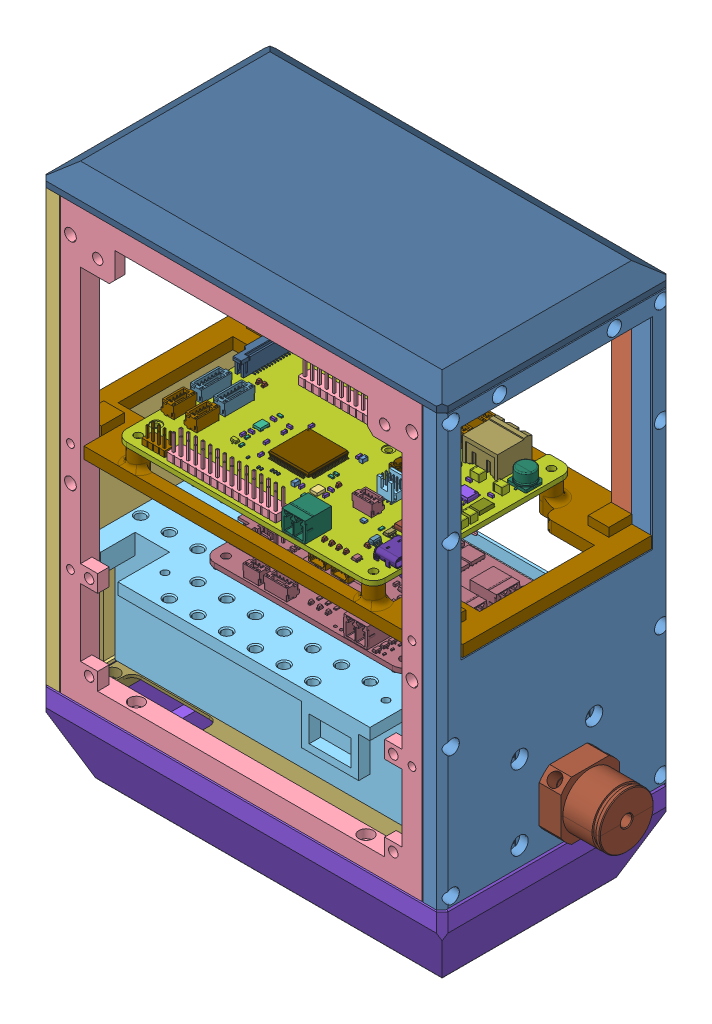
SolidWorks assembly twipr, configuration Default. Lengths in mm. (continued)
Components (placement in the parent): (continued)
- robot-hub-1: robot-hub [Default] at (-323.8774 211.7203 115.5) x (-1 0 0) z (0 1 0) size (91.46 70 13.31) (continued)
  - robot-hub.step-1: robot-hub.step [Default] at origin size (91.46 70 13.31) (continued)
    - R_0603_1608Metric.step-39: R_0603_1608Metric.step [Default] at (94.4 -135.4 -0.05) x (0 -1 0) z (0 0 -1) size (1.6 0.8 0.45) (continued)
      - SOLID.step-1: SOLID.step [Default] at origin size (1.6 0.8 0.45)
    - C_1210_3225Metric.step-7: C_1210_3225Metric.step [Default] at (104.4 -92 -0.05) x (-1 0 0) z (0 0 -1) size (3.2 2.5 2.5)
      - SOLID-0.step-1: SOLID-0.step [Default] at origin size (3.2 2.5 2.5)
    - SOT-323_SC-70.step-3: SOT-323_SC-70.step [Default] at (97 -134 -0.05) x (1 0 0) z (0 0 -1) size (2 2 1.05)
      - SOLID-17.step-1: SOLID-17.step [Default] at origin size (2 2 1.05)
    - SM04B-SRSS-TB_dark.step-2: SM04B-SRSS-TB_dark.step [Default] at (159.3 -135.7 0.2) x (0 -1 0) z (1 0 0) size (6 2.96 4.95)
      - SOLID-37.step-1: SOLID-37.step [Default] at origin size (6 2.96 4.95)
    - C_0603_1608Metric.step-24: C_0603_1608Metric.step [Default] at (116.8 -86.6 -0.05) x (0 -1 0) z (0 0 -1) size (1.6 0.8 0.8)
      - SOLID-1.step-1: SOLID-1.step [Default] at origin size (1.6 0.8 0.8)
    - C_0603_1608Metric.step-25: C_0603_1608Metric.step [Default] at (137.5 -140.9 -0.05) x (0 1 0) z (0 0 -1) size (1.6 0.8 0.8)
      - SOLID-1.step-1: SOLID-1.step [Default] at origin size (1.6 0.8 0.8)
    - C_0805_2012Metric.step-7: C_0805_2012Metric.step [Default] at (85.7 -87.2 -0.05) x (1 0 0) z (0 0 -1) size (2 1.25 1.25)
      - SOLID-11.step-1: SOLID-11.step [Default] at origin size (2 1.25 1.25)
    - IS25LP032D-JNLA3-TR.step-2: IS25LP032D-JNLA3-TR.step [Default] at (144.7 -137.5 -0.05) x (0 -1 0) z (0 0 -1) size (6 4.9 1.75)
      - COMPOUND-21.step-1: COMPOUND-21.step [Default] at origin size (6 4.9 1.75)
    - C_0603_1608Metric.step-26: C_0603_1608Metric.step [Default] at (128 -105.5 -0.05) x (0 1 0) z (0 0 -1) size (1.6 0.8 0.8)
      - SOLID-1.step-1: SOLID-1.step [Default] at origin size (1.6 0.8 0.8)
    - SOT-23-6.step-2: SOT-23-6.step [Default] at (102.8 -123.7 -0.05) x (-1 0 0) z (0 0 -1) size (2.8 2.9 1.55)
      - SOLID-24.step-1: SOLID-24.step [Default] at origin size (2.8 2.9 1.55)
    - PCT2075TP,147.step-1: PCT2075TP,147.step [Default] at (116 -141.3 -0.05) x (0 -1 0) z (0 0 -1) size (3.1 2 0.8)
      - COMPOUND-44.step-1: COMPOUND-44.step [Default] at origin size (3.1 2 0.8)
    - sk6812_side.step-1: sk6812_side.step [Default] at (75.35 -89.1 -1.05) x (0 -1 0) z (-1 0 0) size (4 2 1.6)
      - SOLID-45.step-1: SOLID-45.step [Default] at origin size (4 2 1.6)
    - R_0603_1608Metric.step-40: R_0603_1608Metric.step [Default] at (96 -111.5 -0.05) x (1 0 0) z (0 0 -1) size (1.6 0.8 0.45)
      - SOLID.step-1: SOLID.step [Default] at origin size (1.6 0.8 0.45)
    - R_0603_1608Metric.step-41: R_0603_1608Metric.step [Default] at (77.2 -90.65 -0.05) x (0 1 0) z (0 0 -1) size (1.6 0.8 0.45)
      - SOLID.step-1: SOLID.step [Default] at origin size (1.6 0.8 0.45)
    - C_0603_1608Metric.step-27: C_0603_1608Metric.step [Default] at (105.3 -137.6 -0.05) x (0 1 0) z (0 0 -1) size (1.6 0.8 0.8)
      - SOLID-1.step-1: SOLID-1.step [Default] at origin size (1.6 0.8 0.8)
    - STM32G031G6U6.step-2: STM32G031G6U6.step [Default] at (108.7 -137.5 -0.05) x (1 0 0) z (0 0 -1) size (4.1 4.1 0.6)
      - COMPOUND-31.step-1: COMPOUND-31.step [Default] at origin size (4.1 4.1 0.6)
    - SN74LVC3G17DCTR.step-1: SN74LVC3G17DCTR.step [Default] at (134.75 -142.2 -0.05) x (0 1 0) z (0 0 -1) size (4 2.95 1.3)
      - COMPOUND-46.step-1: COMPOUND-46.step [Default] at origin size (4 2.95 1.3)
    - R_0603_1608Metric.step-42: R_0603_1608Metric.step [Default] at (108.9 -109.7 -0.05) x (-1 0 0) z (0 0 -1) size (1.6 0.8 0.45)
      - SOLID.step-1: SOLID.step [Default] at origin size (1.6 0.8 0.45)
    - C_0805_2012Metric.step-8: C_0805_2012Metric.step [Default] at (94.8 -100.9 -0.05) x (0 1 0) z (0 0 -1) size (2 1.25 1.25)
      - SOLID-11.step-1: SOLID-11.step [Default] at origin size (2 1.25 1.25)
    - M24512-DFDW6TP.step-2: M24512-DFDW6TP.step [Default] at (121.95 -141.55 -0.05) x (1 0 0) z (0 0 -1) size (6.4 3 1.2)
      - COMPOUND-38.step-1: COMPOUND-38.step [Default] at origin size (6.4 3 1.2)
    - C_0603_1608Metric.step-28: C_0603_1608Metric.step [Default] at (101.6 -87.75 -0.05) x (1 0 0) z (0 0 -1) size (1.6 0.8 0.8)
      - SOLID-1.step-1: SOLID-1.step [Default] at origin size (1.6 0.8 0.8)
    - C_0603_1608Metric.step-29: C_0603_1608Metric.step [Default] at (108 -133.3 -0.05) x (0 -1 0) z (0 0 -1) size (1.6 0.8 0.8)
      - SOLID-1.step-1: SOLID-1.step [Default] at origin size (1.6 0.8 0.8)
    - R_0603_1608Metric.step-43: R_0603_1608Metric.step [Default] at (126.9 -130.4 -0.05) x (0 -1 0) z (0 0 -1) size (1.6 0.8 0.45)
      - SOLID.step-1: SOLID.step [Default] at origin size (1.6 0.8 0.45)
    - R_0603_1608Metric.step-44: R_0603_1608Metric.step [Default] at (141.135 -134.9385 -0.05) x (0 1 0) z (0 0 -1) size (1.6 0.8 0.45)
      - SOLID.step-1: SOLID.step [Default] at origin size (1.6 0.8 0.45)
    - SOT-23-6.step-3: SOT-23-6.step [Default] at (153.1 -91.8 -0.05) x (1 0 0) z (0 0 -1) size (2.8 2.9 1.55)
      - SOLID-24.step-1: SOLID-24.step [Default] at origin size (2.8 2.9 1.55)
    - R_0603_1608Metric.step-45: R_0603_1608Metric.step [Default] at (119.59 -119.2 -0.05) x (-1 0 0) z (0 0 -1) size (1.6 0.8 0.45)
      - SOLID.step-1: SOLID.step [Default] at origin size (1.6 0.8 0.45)
    - R_0603_1608Metric.step-46: R_0603_1608Metric.step [Default] at (128.5 -130.4 -0.05) x (0 -1 0) z (0 0 -1) size (1.6 0.8 0.45)
      - SOLID.step-1: SOLID.step [Default] at origin size (1.6 0.8 0.45)
    - R_0603_1608Metric.step-47: R_0603_1608Metric.step [Default] at (128.8 -109 -0.05) x (0 1 0) z (0 0 -1) size (1.6 0.8 0.45)
      - SOLID.step-1: SOLID.step [Default] at origin size (1.6 0.8 0.45)
    - C_0805_2012Metric.step-9: C_0805_2012Metric.step [Default] at (96.9 -100.9 -0.05) x (0 1 0) z (0 0 -1) size (2 1.25 1.25)
      - SOLID-11.step-1: SOLID-11.step [Default] at origin size (2 1.25 1.25)
    - R_0603_1608Metric.step-48: R_0603_1608Metric.step [Default] at (141.135 -138.0385 -0.05) x (0 -1 0) z (0 0 -1) size (1.6 0.8 0.45)
      - SOLID.step-1: SOLID.step [Default] at origin size (1.6 0.8 0.45)
    - SM04B-SRSS-TB_dark.step-3: SM04B-SRSS-TB_dark.step [Default] at (101.5 -142.1 0.2) x (-1 0 0) z (0 -1 0) size (6 2.96 4.95)
      - SOLID-37.step-1: SOLID-37.step [Default] at origin size (6 2.96 4.95)
    - C_0603_1608Metric.step-30: C_0603_1608Metric.step [Default] at (139.0125 -133.3 -0.05) x (0 1 0) z (0 0 -1) size (1.6 0.8 0.8)
      - SOLID-1.step-1: SOLID-1.step [Default] at origin size (1.6 0.8 0.8)
    - R_0603_1608Metric.step-49: R_0603_1608Metric.step [Default] at (152.7 -142.2 -0.05) x (1 0 0) z (0 0 -1) size (1.6 0.8 0.45)
      - SOLID.step-1: SOLID.step [Default] at origin size (1.6 0.8 0.45)
    - C_0805_2012Metric.step-10: C_0805_2012Metric.step [Default] at (85.75 -93.75 -0.05) x (1 0 0) z (0 0 -1) size (2 1.25 1.25)
      - SOLID-11.step-1: SOLID-11.step [Default] at origin size (2 1.25 1.25)
    - R_0603_1608Metric.step-50: R_0603_1608Metric.step [Default] at (127.7 -96.9 -0.05) x (1 0 0) z (0 0 -1) size (1.6 0.8 0.45)
      - SOLID.step-1: SOLID.step [Default] at origin size (1.6 0.8 0.45)
    - C_0805_2012Metric.step-11: C_0805_2012Metric.step [Default] at (100.75 -132.4 -0.05) x (1 0 0) z (0 0 -1) size (2 1.25 1.25)
      - SOLID-11.step-1: SOLID-11.step [Default] at origin size (2 1.25 1.25)
    - NCV8187AMLE330TCG.step-1: NCV8187AMLE330TCG.step [Default] at (96.2 -119.9 -0.05) x (-1 0 0) z (0 0 -1) size (3.1 3 1)
      - COMPOUND-47.step-1: COMPOUND-47.step [Default] at origin size (3.1 3 1)
    - R_0402_1005Metric.step-11: R_0402_1005Metric.step [Default] at (91.95 -87.35 -0.05) x (-1 0 0) z (0 0 -1) size (1 0.5 0.35)
      - SOLID-3.step-1: SOLID-3.step [Default] at origin size (1 0.5 0.35)
    - SOIC-16_3.9x9.9mm_P1.27mm.step-1: SOIC-16_3.9x9.9mm_P1.27mm.step [Default] at (96.9 -106.7 -0.05) x (0 1 0) z (0 0 -1) size (6 9.9 1.75)
      - SOLID-48.step-1: SOLID-48.step [Default] at origin size (6 9.9 1.75)
    - C_0603_1608Metric.step-31: C_0603_1608Metric.step [Default] at (96.8 -92.75 -0.05) x (-1 0 0) z (0 0 -1) size (1.6 0.8 0.8)
      - SOLID-1.step-1: SOLID-1.step [Default] at origin size (1.6 0.8 0.8)
    - R_0603_1608Metric.step-51: R_0603_1608Metric.step [Default] at (107.7 -107.2 -0.05) x (0 1 0) z (0 0 -1) size (1.6 0.8 0.45)
      - SOLID.step-1: SOLID.step [Default] at origin size (1.6 0.8 0.45)
    - R_0603_1608Metric.step-52: R_0603_1608Metric.step [Default] at (141.5 -130.7 -0.05) x (0 -1 0) z (0 0 -1) size (1.6 0.8 0.45)
      - SOLID.step-1: SOLID.step [Default] at origin size (1.6 0.8 0.45)
    - ECS-120-20-33-CKM-TR.step-1: ECS-120-20-33-CKM-TR.step [Default] at (104.7 -102.5 -0.05) x (0 1 0) z (0 0 -1) size (3.38 2.68 0.9)
      - COMPOUND-49.step-1: COMPOUND-49.step [Default] at origin size (3.38 2.68 0.9)
    - R_0603_1608Metric.step-53: R_0603_1608Metric.step [Default] at (93.5 -139.3 -0.05) x (0 -1 0) z (0 0 -1) size (1.6 0.8 0.45)
      - SOLID.step-1: SOLID.step [Default] at origin size (1.6 0.8 0.45)
    - C_0603_1608Metric.step-32: C_0603_1608Metric.step [Default] at (125.4 -99.5 -0.05) x (0 1 0) z (0 0 -1) size (1.6 0.8 0.8)
      - SOLID-1.step-1: SOLID-1.step [Default] at origin size (1.6 0.8 0.8)
    - R_0402_1005Metric.step-12: R_0402_1005Metric.step [Default] at (91.95 -88.35 -0.05) x (1 0 0) z (0 0 -1) size (1 0.5 0.35)
      - SOLID-3.step-1: SOLID-3.step [Default] at origin size (1 0.5 0.35)
    - 5033981892.step-1: 5033981892.step [Default] at (97.05 29.65 -154.55) x (0 -1 0) z (0 0 1) size (13.1 14.05 1.28)
      - COMPOUND-50.step-1: COMPOUND-50.step [Default] at origin size (13.1 14.05 1.28)
    - R_0603_1608Metric.step-54: R_0603_1608Metric.step [Default] at (131.9625 -136.35 -0.05) x (0 -1 0) z (0 0 -1) size (1.6 0.8 0.45)
      - SOLID.step-1: SOLID.step [Default] at origin size (1.6 0.8 0.45)
    - SOT-563.step-2: SOT-563.step [Default] at (89.5 -84.65 -0.05) x (-1 0 0) z (0 0 -1) size (1.6 1.6 0.63)
      - SOLID-29.step-1: SOLID-29.step [Default] at origin size (1.6 1.6 0.63)
    - R_0603_1608Metric.step-55: R_0603_1608Metric.step [Default] at (94.45 -93.2 -0.05) x (0 -1 0) z (0 0 -1) size (1.6 0.8 0.45)
      - SOLID.step-1: SOLID.step [Default] at origin size (1.6 0.8 0.45)
    - R_0603_1608Metric.step-56: R_0603_1608Metric.step [Default] at (123.9 -130.4 -0.05) x (0 -1 0) z (0 0 -1) size (1.6 0.8 0.45)
      - SOLID.step-1: SOLID.step [Default] at origin size (1.6 0.8 0.45)
    - R_0603_1608Metric.step-57: R_0603_1608Metric.step [Default] at (117 -100 -0.05) x (0 -1 0) z (0 0 -1) size (1.6 0.8 0.45)
      - SOLID.step-1: SOLID.step [Default] at origin size (1.6 0.8 0.45)
    - R_0603_1608Metric.step-58: R_0603_1608Metric.step [Default] at (91.7 -139.3 -0.05) x (0 -1 0) z (0 0 -1) size (1.6 0.8 0.45)
      - SOLID.step-1: SOLID.step [Default] at origin size (1.6 0.8 0.45)
    - R_0402_1005Metric.step-13: R_0402_1005Metric.step [Default] at (91.95 -89.35 -0.05) x (1 0 0) z (0 0 -1) size (1 0.5 0.35)
      - SOLID-3.step-1: SOLID-3.step [Default] at origin size (1 0.5 0.35)
    - sk6812_side.step-2: sk6812_side.step [Default] at (75.35 -96.1 -1.05) x (0 -1 0) z (-1 0 0) size (4 2 1.6)
      - SOLID-45.step-1: SOLID-45.step [Default] at origin size (4 2 1.6)
    - R_0603_1608Metric.step-59: R_0603_1608Metric.step [Default] at (118.6 -100 -0.05) x (0 -1 0) z (0 0 -1) size (1.6 0.8 0.45)
      - SOLID.step-1: SOLID.step [Default] at origin size (1.6 0.8 0.45)
    - C_0805_2012Metric.step-12: C_0805_2012Metric.step [Default] at (92.9 -119.9 -0.05) x (0 -1 0) z (0 0 -1) size (2 1.25 1.25)
      - SOLID-11.step-1: SOLID-11.step [Default] at origin size (2 1.25 1.25)
    - C_0805_2012Metric.step-13: C_0805_2012Metric.step [Default] at (103.5 -135.8 -0.05) x (0 1 0) z (0 0 -1) size (2 1.25 1.25)
      - SOLID-11.step-1: SOLID-11.step [Default] at origin size (2 1.25 1.25)
    - SM04B-SRSS-TB_dark.step-4: SM04B-SRSS-TB_dark.step [Default] at (159.3 -127.9 0.2) x (0 -1 0) z (1 0 0) size (6 2.96 4.95)
      - SOLID-37.step-1: SOLID-37.step [Default] at origin size (6 2.96 4.95)
    - C_0603_1608Metric.step-33: C_0603_1608Metric.step [Default] at (78.75 -90.65 -0.05) x (0 1 0) z (0 0 -1) size (1.6 0.8 0.8)
      - SOLID-1.step-1: SOLID-1.step [Default] at origin size (1.6 0.8 0.8)
    - SN74LVC3G17DCTR.step-2: SN74LVC3G17DCTR.step [Default] at (134.7125 -134.9 -0.05) x (0 1 0) z (0 0 -1) size (4 2.95 1.3)
      - COMPOUND-46.step-1: COMPOUND-46.step [Default] at origin size (4 2.95 1.3)
    - DMS0008A.step-1: DMS0008A.step [Default] at (85.1 -135.6 -0.05) x (-1 0 0) z (0 0 -1) size (3.3 3.3 0.8)
      - COMPOUND-51.step-1: COMPOUND-51.step [Default] at origin size (3.3 3.3 0.8)
    - TPS22975NDSGT.step-1: TPS22975NDSGT.step [Default] at (104.8 -88.5 -0.05) x (0 1 0) z (0 0 -1) size (2 2 0.78)
      - COMPOUND-52.step-1: COMPOUND-52.step [Default] at origin size (2 2 0.78)
    - R_0603_1608Metric.step-60: R_0603_1608Metric.step [Default] at (143.1 -130.7 -0.05) x (0 -1 0) z (0 0 -1) size (1.6 0.8 0.45)
      - SOLID.step-1: SOLID.step [Default] at origin size (1.6 0.8 0.45)
    - Fuse_1206_3216Metric.step-2: Fuse_1206_3216Metric.step [Default] at (107.4 -86.4 -0.05) x (0 1 0) z (0 0 -1) size (3.2 1.6 0.55)
      - SOLID-32.step-1: SOLID-32.step [Default] at origin size (3.2 1.6 0.55)
    - SM04B-SRSS-TB_dark.step-5: SM04B-SRSS-TB_dark.step [Default] at (94 -81 0.2) x (1 0 0) z (0 1 0) size (6 2.96 4.95)
      - SOLID-37.step-1: SOLID-37.step [Default] at origin size (6 2.96 4.95)
    - R_0603_1608Metric.step-61: R_0603_1608Metric.step [Default] at (115.7 -89.4 -0.05) x (-1 0 0) z (0 0 -1) size (1.6 0.8 0.45)
      - SOLID.step-1: SOLID.step [Default] at origin size (1.6 0.8 0.45)
    - R_0603_1608Metric.step-62: R_0603_1608Metric.step [Default] at (101.2 -129.6 -0.05) x (0 -1 0) z (0 0 -1) size (1.6 0.8 0.45)
      - SOLID.step-1: SOLID.step [Default] at origin size (1.6 0.8 0.45)
    - R_0603_1608Metric.step-63: R_0603_1608Metric.step [Default] at (148.335 -138.0385 -0.05) x (0 1 0) z (0 0 -1) size (1.6 0.8 0.45)
      - SOLID.step-1: SOLID.step [Default] at origin size (1.6 0.8 0.45)
    - PCT2075TP,147.step-2: PCT2075TP,147.step [Default] at (125 -105.6 -0.05) x (1 0 0) z (0 0 -1) size (3.1 2 0.8)
      - COMPOUND-44.step-1: COMPOUND-44.step [Default] at origin size (3.1 2 0.8)
    - R_0603_1608Metric.step-64: R_0603_1608Metric.step [Default] at (101.6 -89.35 -0.05) x (1 0 0) z (0 0 -1) size (1.6 0.8 0.45)
      - SOLID.step-1: SOLID.step [Default] at origin size (1.6 0.8 0.45)
    - R_0603_1608Metric.step-65: R_0603_1608Metric.step [Default] at (149.6 -109.1 -0.05) x (0 -1 0) z (0 0 -1) size (1.6 0.8 0.45)
      - SOLID.step-1: SOLID.step [Default] at origin size (1.6 0.8 0.45)
    - R_0603_1608Metric.step-66: R_0603_1608Metric.step [Default] at (153 -84.3 -0.05) x (0 1 0) z (0 0 -1) size (1.6 0.8 0.45)
      - SOLID.step-1: SOLID.step [Default] at origin size (1.6 0.8 0.45)
    - C_0603_1608Metric.step-34: C_0603_1608Metric.step [Default] at (132 -140.4 -0.05) x (0 1 0) z (0 0 -1) size (1.6 0.8 0.8)
      - SOLID-1.step-1: SOLID-1.step [Default] at origin size (1.6 0.8 0.8)
    - C_0603_1608Metric.step-35: C_0603_1608Metric.step [Default] at (151.45 -132.75 -0.05) x (-1 0 0) z (0 0 -1) size (1.6 0.8 0.8)
      - SOLID-1.step-1: SOLID-1.step [Default] at origin size (1.6 0.8 0.8)
    - R_0603_1608Metric.step-67: R_0603_1608Metric.step [Default] at (101.4 -101.2 -0.05) x (0 1 0) z (0 0 -1) size (1.6 0.8 0.45)
      - SOLID.step-1: SOLID.step [Default] at origin size (1.6 0.8 0.45)
    - R_0603_1608Metric.step-68: R_0603_1608Metric.step [Default] at (108.9 -111.2 -0.05) x (-1 0 0) z (0 0 -1) size (1.6 0.8 0.45)
      - SOLID.step-1: SOLID.step [Default] at origin size (1.6 0.8 0.45)
    - Fuse_1206_3216Metric.step-3: Fuse_1206_3216Metric.step [Default] at (90.5 -120.5 -0.05) x (0 -1 0) z (0 0 -1) size (3.2 1.6 0.55)
      - SOLID-32.step-1: SOLID-32.step [Default] at origin size (3.2 1.6 0.55)
    - robot-hub_rev3 PCB.step-1: robot-hub_rev3 PCB.step [Default] at origin size (90 70 1.66)
- bat_compartment-1: bat_compartment [Default] at (-442.6774 127.2203 0) x (-1 0 0) z (0 0 1) size (140 30 80)
- platform_control-1: platform_control [Default] at (-442.6774 200.7203 -0.1) size (140 11 78)
- marker_top-1: marker_top [Default] at (-442.6774 277.2203 0) size (140 14 80)
- T81H-RM41.stp-1: T81H-RM41.stp [Default] at (-368.6774 147.2203 0) x (0 0 -1) z (1 0 0) size (20.32 20.32 20.32)
- T81H-RM41.stp-2: T81H-RM41.stp [Default] at (-516.6774 147.2203 0) x (0 0 1) z (-1 0 0) size (20.32 20.32 20.32)
- bat_compartment_lid-1: bat_compartment_lid [Default] at (-442.6774 127.2203 0) x (-1 0 0) z (0 0 1) size (125.4 4 62)
- SimpleBMS-1: SimpleBMS [Default] at (-264.9746 172.7203 56) x (-1 0 0) z (0 1 0) size (70 50 11.7)
- cover_1-1: cover_1 [Default] at (-442.6774 151.9703 40) x (-1 0 0) z (0 0 -1) size (111.2 35.5 3) (hidden)
- cover_2-1: cover_2 [Default] at (-442.6774 151.9703 -40) size (111.2 35.5 3) (hidden)
- SE020A_01a-1: SE020A_01a [Default] at (-382.6774 147.2203 0) x (0 1 0) z (0 0 1) size (35.71 70 44.21)
- SE020A_01a-2: SE020A_01a [Default] at (-502.6774 147.2203 0) x (0 -1 0) z (0 0 1) size (35.71 70 44.21)
Mates (geometry in assembly coordinates):
- Parallel1: parallel anti-aligned: plane of brace_left-1 through (-379.6774 202.2203 0) normal (-1 0 0)
- Coincident4: coincident anti-aligned: plane of brace_left-1 through (-379.6774 202.2203 0) normal (0 0 -1)
- Coincident5: coincident aligned: plane of brace_left-1 through (-372.6774 127.2203 -40) normal (0 0 -1); plane of brace_front-1 through (-442.6774 202.2203 -40) normal (0 0 -1)
- Coincident6: coincident aligned: plane of brace_left-1 through (-372.6774 277.2203 40) normal (0 1 0); plane of brace_front-1 through (-505.6774 277.2203 -33) normal (0 1 0)
- Coincident7: coincident anti-aligned: plane of brace_left-1 through (-379.6774 202.2203 0) normal (-1 0 0); plane of brace_front-1 through (-379.6774 127.2203 -33) normal (1 0 0)
- Coincident8: coincident anti-aligned: plane of brace_front-1 through (-505.6774 127.2203 -33) normal (-1 0 0); plane of brace_right-1 through (-505.6774 202.2203 0) normal (1 0 0)
- Coincident9: coincident aligned: plane of brace_front-1 through (-505.6774 277.2203 -33) normal (0 1 0); plane of brace_right-1 through (-512.6774 277.2203 -40) normal (0 1 0)
- Coincident10: coincident aligned: plane of brace_front-1 through (-442.6774 202.2203 -40) normal (0 0 -1); plane of brace_right-1 through (-512.6774 127.2203 -40) normal (0 0 -1)
- Coincident11: coincident anti-aligned: plane of brace_left-1 through (-379.6774 202.2203 0) normal (-1 0 0); plane of brace_back-1 through (-379.6774 127.2203 40) normal (1 0 0)
- Coincident12: coincident aligned: plane of brace_left-1 through (-372.6774 277.2203 40) normal (0 1 0); plane of brace_back-1 through (-505.6774 277.2203 40) normal (0 1 0)
- Coincident13: coincident aligned: plane of brace_left-1 through (-372.6774 127.2203 40) normal (0 0 1); plane of brace_back-1 through (-442.6774 202.2203 40) normal (0 0 1)
- Parallel5: parallel anti-aligned: plane of brace_left-1 through (-372.6774 202.2203 0) normal (1 0 0); plane of banebots_4_78-1 through (-361.252 137.0603 10.16) normal (-1 0 0)
- Coincident25: coincident anti-aligned: plane of banebots_4_78-1 through (-368.872 147.2203 0) normal (0 0 -1)
- Coincident26: coincident aligned: plane of banebots_4_78-1 through (-368.872 147.2203 0) normal (0 1 0); plane of banebots_4_78-2 through (-516.2261 147.2203 0) normal (0 1 0)
- Coincident27: coincident anti-aligned: plane of banebots_4_78-1 through (-368.872 147.2203 0) normal (0 0 -1); plane of banebots_4_78-2 through (-516.2261 147.2203 0) normal (0 0 1)
- Coincident31: coincident anti-aligned: plane of brace_back-1 through (-505.6774 127.2203 40) normal (0 -1 0); plane of bat_compartment-1 through (-442.6774 127.2203 0) normal (0 1 0)
- Coincident32: coincident aligned: plane of brace_back-1 through (-442.6774 202.2203 40) normal (0 0 1); plane of bat_compartment-1 through (-372.6774 120.2203 40) normal (0 0 1)
- Coincident33: coincident aligned: plane of brace_left-1 through (-372.6774 202.2203 0) normal (1 0 0); plane of bat_compartment-1 through (-372.6774 120.2203 40) normal (1 0 0)
- Coincident36: coincident aligned: plane of brace_right-1 through (-512.6774 202.2203 0) normal (-1 0 0); plane of platform_control-1 through (-512.6774 204.7203 32.8) normal (-1 0 0)
- Coincident38: coincident anti-aligned: plane of brace_left-1 through (-372.6774 277.2203 40) normal (0 1 0); plane of marker_top-1 through (-442.6774 277.2203 0) normal (0 -1 0)
- Coincident39: coincident aligned: plane of brace_front-1 through (-442.6774 202.2203 -40) normal (0 0 -1); plane of marker_top-1 through (-512.6774 279.2203 -40) normal (0 0 -1)
- Coincident40: coincident aligned: plane of brace_right-1 through (-512.6774 202.2203 0) normal (-1 0 0); plane of marker_top-1 through (-512.6774 279.2203 40) normal (-1 0 0)
- Coincident42: coincident anti-aligned: plane of robot-hub-1/robot-hub.step-1/robot-hub_rev3 PCB.step-1 through (-441.9229 211.7203 3.2681) normal (0 -1 0); plane of platform_control-1 through (-483.6774 211.7203 34.9) normal (0 1 0)
- Concentric7: concentric aligned: circle of robot-hub-1/robot-hub.step-1/robot-hub_rev3 PCB.step-1; circle of platform_control-1
- Concentric8: concentric aligned: circle of robot-hub-1/robot-hub.step-1/robot-hub_rev3 PCB.step-1; circle of platform_control-1
- Concentric11: concentric aligned: circle of brace_front-1; circle of platform_control-1
- Concentric274: concentric aligned: circle of brace_front-1; circle of platform_middle-1
- Coincident583: coincident aligned: plane of brace_left-1 through (-379.6774 202.2203 0) normal (0 0 -1); plane of T81H-RM41.stp-1 through (-368.6774 147.2203 0) normal (0 0 -1)
- Distance2: distance = 4 mm: point of T81H-RM41.stp-1; plane of brace_left-1 through (-372.6774 202.2203 0) normal (1 0 0)
- Coincident586: coincident aligned: plane of brace_right-1 through (-505.6774 202.2203 0) normal (0 0 1); plane of T81H-RM41.stp-2 through (-516.6774 147.2203 0) normal (0 0 1)
- Distance3: distance = 4 mm: point of T81H-RM41.stp-2; plane of brace_right-1 through (-512.6774 202.2203 0) normal (-1 0 0)
- Lock1: lock: unknown of banebots_4_78-1; unknown of T81H-RM41.stp-1
- Lock2: lock: unknown of banebots_4_78-2; unknown of T81H-RM41.stp-2
- Coincident591: coincident anti-aligned: plane of brace_back-1 through (-442.6774 202.2203 33) normal (0 0 -1); plane of platform_middle-1 through (-505.7274 169.7203 33) normal (0 0 1)
- Coincident592: coincident anti-aligned: plane of brace_front-1 through (-442.6774 202.2203 -33) normal (0 0 1); plane of platform_control-1 through (-512.6774 204.7203 -33) normal (0 0 -1)
- Coincident593: coincident anti-aligned: plane of bat_compartment-1 through (-442.6774 123.2203 0) normal (0 1 0); plane of bat_compartment_lid-1 through (-442.6774 123.2203 0) normal (0 -1 0)
- Concentric275: concentric aligned: circle of bat_compartment-1; circle of bat_compartment_lid-1
- Concentric276: concentric aligned: circle of bat_compartment-1; circle of bat_compartment_lid-1
- Coincident597: coincident anti-aligned: plane of brace_front-1 through (-442.6774 202.2203 -37) normal (0 0 -1); plane of cover_2-1 through (-442.6774 151.9703 -37) normal (0 0 1)
- Concentric279: concentric anti-aligned: circle of brace_front-1; circle of cover_2-1
- Concentric280: concentric anti-aligned: circle of brace_front-1; cylinder of cover_2-1 through (-389.6774 166.7203 -40) axis (0 0 1) radius 1.1
- Parallel8: parallel anti-aligned: plane of brace_left-1 through (-379.6774 202.2203 0) normal (-1 0 0); plane of platform_middle-1 through (-379.7274 169.7203 33) normal (1 0 0)
- Coincident598: coincident anti-aligned: plane of brace_left-1 through (-378.6774 202.2203 0) normal (-1 0 0); plane of SE020A_01a-1 through (-378.6774 147.2203 -1) normal (1 0 0)
- Concentric281: concentric aligned: circle of brace_left-1; circle of SE020A_01a-1
- Parallel9: parallel aligned: plane of platform_middle-1 through (-462.7274 87.6703 -21.5) normal (0 0 -1); plane of SE020A_01a-1 through (-403.6774 147.2203 -21.5) normal (0 0 -1)
- Coincident600: coincident anti-aligned: plane of brace_right-1 through (-506.6774 202.2203 0) normal (1 0 0); plane of SE020A_01a-2 through (-506.6774 147.2203 -1) normal (-1 0 0)
- Concentric282: concentric aligned: circle of brace_right-1; circle of SE020A_01a-2
- Parallel10: parallel aligned: plane of platform_middle-1 through (-462.7274 87.6703 -21.5) normal (0 0 -1); plane of SE020A_01a-2 through (-481.6774 147.2203 -21.5) normal (0 0 -1)
